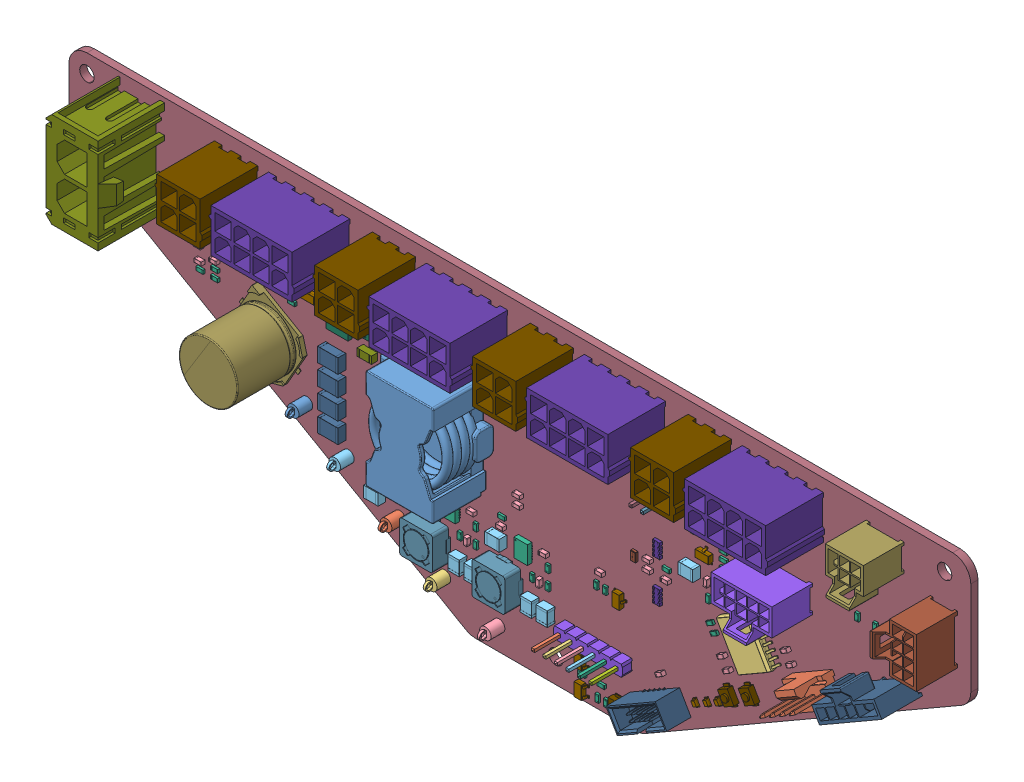
SolidWorks assembly zaphod-controller, configuration Default. Lengths in mm.
Overall size (199.92 69.34 18.57).
449 component instances, 49 part files, 0 mates.
Components (placement in the parent):
- PKMCS0909E4000-1: PKMCS0909E4000 [Default] at (113.5 -47 -0.05) x (-1 0 0) z (0 -1 0) size (9 1.9 9)
  - COMPOUND-1: COMPOUND [Default] at origin size (9 1.9 9)
- MOLEX_47053-1000-1: MOLEX_47053-1000 [Default] at (166.5524 -41.075 4.15) x (0.866025 0.5 0) z (0.5 -0.866025 0) size (10.2 13.5 5.84)
  - SOLID-1: SOLID [Default] at origin size (10.2 13.5 5.84)
- SOIC127P1032X265-16L87-1: SOIC127P1032X265-16L87 [Default] at (151.3126 -39.0334 1.65) x (0.5 -0.866025 0) z (0 0 1) size (10.08 10.17 2)
  - COMPOUND_2-1: COMPOUND_2 [Default] at origin size (10.08 10.17 2)
- CAPC1608X90-1: CAPC1608X90 [Default] at (147.0091 -44.05 -0.05) x (0 -1 0) z (0 0 -1) size (1.6 0.8 0.9)
  - COMPOUND_3-1: COMPOUND_3 [Default] at origin size (1.6 0.8 0.9)
- CAPC1608X90-2: CAPC1608X90 [Default] at (147.1 -51.575 -0.05) x (0 -1 0) z (0 0 -1) size (1.6 0.8 0.9)
  - COMPOUND_3-1: COMPOUND_3 [Default] at origin size (1.6 0.8 0.9)
- CAPC1608X90-3: CAPC1608X90 [Default] at (134.6 -51.575 -0.05) x (0 -1 0) z (0 0 -1) size (1.6 0.8 0.9)
  - COMPOUND_3-1: COMPOUND_3 [Default] at origin size (1.6 0.8 0.9)
- CAPC1608X90-4: CAPC1608X90 [Default] at (134.6 -45.075 -0.05) x (0 -1 0) z (0 0 -1) size (1.6 0.8 0.9)
  - COMPOUND_3-1: COMPOUND_3 [Default] at origin size (1.6 0.8 0.9)
- CAPC1608X90-5: CAPC1608X90 [Default] at (145.2978 -44.8154 1.65) x (0.866025 0.5 0) z (0 0 1) size (1.6 0.8 0.9)
  - COMPOUND_3-1: COMPOUND_3 [Default] at origin size (1.6 0.8 0.9)
- CAPC1608X90-6: CAPC1608X90 [Default] at (160.5774 -38.8805 1.65) x (-0.866025 -0.5 0) z (0 0 1) size (1.6 0.8 0.9)
  - COMPOUND_3-1: COMPOUND_3 [Default] at origin size (1.6 0.8 0.9)
- CAPC3225X170-1: CAPC3225X170 [Default] at (153.35 -43.55 -0.05) x (0 -1 0) z (0 0 -1) size (3.2 2.5 1.7)
  - COMPOUND_4-1: COMPOUND_4 [Default] at origin size (3.2 2.5 1.7)
- CAPC3225X170-2: CAPC3225X170 [Default] at (131.85 -44.325 -0.05) x (0 -1 0) z (0 0 -1) size (3.2 2.5 1.7)
  - COMPOUND_4-1: COMPOUND_4 [Default] at origin size (3.2 2.5 1.7)
- RESC1608X50-1: RESC1608X50 [Default] at (157.1 -45.05 -0.05) x (1 0 0) z (0 0 -1) size (1.6 0.8 0.5)
  - COMPOUND_5-1: COMPOUND_5 [Default] at origin size (1.6 0.8 0.5)
- RESC1608X50-2: RESC1608X50 [Default] at (156.5275 -31.8657 1.65) x (-0.866025 -0.5 0) z (0 0 1) size (1.6 0.8 0.5)
  - COMPOUND_5-1: COMPOUND_5 [Default] at origin size (1.6 0.8 0.5)
- RESC1608X50-3: RESC1608X50 [Default] at (157.1 -43.3 -0.05) x (1 0 0) z (0 0 -1) size (1.6 0.8 0.5)
  - COMPOUND_5-1: COMPOUND_5 [Default] at origin size (1.6 0.8 0.5)
- RESC1608X50-4: RESC1608X50 [Default] at (157.4525 -33.4678 1.65) x (-0.866025 -0.5 0) z (0 0 1) size (1.6 0.8 0.5)
  - COMPOUND_5-1: COMPOUND_5 [Default] at origin size (1.6 0.8 0.5)
- SOP65P780X200-24L40-1: SOP65P780X200-24L40 [Default] at (140.85 -47.8 -0.25) x (1 0 0) z (0 1 0) size (7.9 2.02 8.63)
  - SOLID_2-1: SOLID_2 [Default] at origin size (7.9 2.02 8.63)
- MOLEX_NANOFIT_1053101110-1: MOLEX_NANOFIT_1053101110 [Default] at (158.2 -24.35 6.5) x (-1 0 0) z (0 0 1) size (13.44 8.86 13.71)
  - SOLID_3-1: SOLID_3 [Default] at origin size (13.44 8.86 13.71)
- SOT95P240X110-3L16-1: SOT95P240X110-3L16 [Default] at (179 -22.5 -0.05) x (0 1 0) z (0 0 -1) size (2.91 3.01 1.23)
  - COMPOUND_6-1: COMPOUND_6 [Default] at origin size (2.91 3.01 1.23)
- RESC1608X50-5: RESC1608X50 [Default] at (182.7 -19.3 -0.05) x (-1 0 0) z (0 0 -1) size (1.6 0.8 0.5)
  - COMPOUND_5-1: COMPOUND_5 [Default] at origin size (1.6 0.8 0.5)
- MOLEX_NANOFIT_1053091106-1: MOLEX_NANOFIT_1053091106 [Default] at (181.5175 -33.225 6.5) x (0.866025 0.5 0) z (0 0 1) size (15.94 6.34 13.71)
  - SOLID_4-1: SOLID_4 [Default] at origin size (15.94 6.34 13.71)
- MOLEX_NANOFIT_1053101108-1: MOLEX_NANOFIT_1053101108 [Default] at (194.05 -16.05 6.55) x (0 1 0) z (0 0 1) size (10.94 8.84 13.71)
  - SOLID_5-1: SOLID_5 [Default] at origin size (10.94 8.84 13.71)
- MOLEX_NANOFIT_1053101106-1: MOLEX_NANOFIT_1053101106 [Default] at (181 -6.25 6.5) x (-1 0 0) z (0 0 1) size (8.44 8.84 13.71)
  - SOLID_6-1: SOLID_6 [Default] at origin size (8.44 8.84 13.71)
- 61300211121-1: 61300211121 [Default] at (133.83 -18.6 2.65) x (1 0 0) z (0 -1 0) size (5.08 11.54 2.54)
  - SOLID_7-1: SOLID_7 [Default] at origin size (0.64 11.54 0.64)
  - SOLID_8-1: SOLID_8 [Default] at origin size (0.64 11.54 0.64)
  - SOLID_9-1: SOLID_9 [Default] at origin size (5.08 2.54 2.54)
- RESC1608X50-6: RESC1608X50 [Default] at (132.8 -34.6 1.65) x (-1 0 0) z (0 0 1) size (1.6 0.8 0.5)
  - COMPOUND_5-1: COMPOUND_5 [Default] at origin size (1.6 0.8 0.5)
- RESC1608X50-7: RESC1608X50 [Default] at (133.8 -21.4 1.65) x (-1 0 0) z (0 0 1) size (1.6 0.8 0.5)
  - COMPOUND_5-1: COMPOUND_5 [Default] at origin size (1.6 0.8 0.5)
- RESC1608X50-8: RESC1608X50 [Default] at (57.7 -27.2 -0.05) x (1 0 0) z (0 0 -1) size (1.6 0.8 0.5)
  - COMPOUND_5-1: COMPOUND_5 [Default] at origin size (1.6 0.8 0.5)
- MOLEX_SABRE_431600102-1: MOLEX_SABRE_431600102 [Default] at (15.5 -11.45 9.05) x (0 1 0) z (1 0 0) size (21.08 18.57 13.39)
  - SOLID_10-1: SOLID_10 [Default] at origin size (21.08 18.57 13.39)
- MOLEX_MICROFITJR_039281083-1: MOLEX_MICROFITJR_039281083 [Default] at (53.3 -7.5 1.65) x (-1 0 0) z (0 1 0) size (18.8 16.3 11)
  - SOLID_11-1: SOLID_11 [Default] at origin size (18.8 16.3 11)
- MOLEX_MICROFITJR_039281083-2: MOLEX_MICROFITJR_039281083 [Default] at (88.3 -7.5 1.65) x (-1 0 0) z (0 1 0) size (18.8 16.3 11)
  - SOLID_11-1: SOLID_11 [Default] at origin size (18.8 16.3 11)
- MOLEX_MICROFITJR_039281083-3: MOLEX_MICROFITJR_039281083 [Default] at (123.3 -7.5 1.65) x (-1 0 0) z (0 1 0) size (18.8 16.3 11)
  - SOLID_11-1: SOLID_11 [Default] at origin size (18.8 16.3 11)
- MOLEX_MICROFITJR_039281083-4: MOLEX_MICROFITJR_039281083 [Default] at (158.3 -7.5 1.65) x (-1 0 0) z (0 1 0) size (18.8 16.3 11)
  - SOLID_11-1: SOLID_11 [Default] at origin size (18.8 16.3 11)
- MOLEX_MICROFITJR_039281043-1: MOLEX_MICROFITJR_039281043 [Default] at (37.1 -7.5 1.65) x (-1 0 0) z (0 1 0) size (10.4 16.3 11)
  - SOLID_12-1: SOLID_12 [Default] at origin size (10.4 16.3 11)
- MOLEX_MICROFITJR_039281043-2: MOLEX_MICROFITJR_039281043 [Default] at (72.1 -7.5 1.65) x (-1 0 0) z (0 1 0) size (10.4 16.3 11)
  - SOLID_12-1: SOLID_12 [Default] at origin size (10.4 16.3 11)
- MOLEX_MICROFITJR_039281043-3: MOLEX_MICROFITJR_039281043 [Default] at (107.1 -7.5 1.65) x (-1 0 0) z (0 1 0) size (10.4 16.3 11)
  - SOLID_12-1: SOLID_12 [Default] at origin size (10.4 16.3 11)
- MOLEX_MICROFITJR_039281043-4: MOLEX_MICROFITJR_039281043 [Default] at (142.1 -7.5 1.65) x (-1 0 0) z (0 1 0) size (10.4 16.3 11)
  - SOLID_12-1: SOLID_12 [Default] at origin size (10.4 16.3 11)
- PULSE_PA2050-1: PULSE_PA2050 [Default] at (84.85 -28.9 1.65) x (0 -1 0) z (-1 0 0) size (22.23 12.2 19.25)
  - SOLID_13-1: SOLID_13 [Default] at origin size (22.23 12.2 19.25)
- 61300611121-1: 61300611121 [Default] at (117.35 -57.1 2.65) x (1 0 0) z (0 -1 0) size (15.24 11.54 2.54)
  - SOLID_14-1: SOLID_14 [Default] at origin size (0.64 11.54 0.64)
  - SOLID_15-1: SOLID_15 [Default] at origin size (0.64 11.54 0.64)
  - SOLID_16-1: SOLID_16 [Default] at origin size (0.64 11.54 0.64)
  - SOLID_17-1: SOLID_17 [Default] at origin size (0.64 11.54 0.64)
  - SOLID_18-1: SOLID_18 [Default] at origin size (0.64 11.54 0.64)
  - SOLID_19-1: SOLID_19 [Default] at origin size (0.64 11.54 0.64)
  - SOLID_20-1: SOLID_20 [Default] at origin size (15.24 2.54 2.54)
- LEDC1608X80L40-1: LEDC1608X80L40 [Default] at (141.8 -55.6 1.75) x (-0.5 0.866025 0) z (0.866025 0.5 0) size (1.61 0.75 0.81)
  - COMPOUND_7-1: COMPOUND_7 [Default] at origin size (1.61 0.75 0.81)
- LEDC1608X80L40-2: LEDC1608X80L40 [Default] at (139.2 -57 1.75) x (-0.5 0.866025 0) z (0.866025 0.5 0) size (1.61 0.75 0.81)
  - COMPOUND_7-1: COMPOUND_7 [Default] at origin size (1.61 0.75 0.81)
- LEDC1608X80L40-3: LEDC1608X80L40 [Default] at (144.2 -54.3 1.75) x (-0.5 0.866025 0) z (0.866025 0.5 0) size (1.61 0.75 0.81)
  - COMPOUND_7-1: COMPOUND_7 [Default] at origin size (1.61 0.75 0.81)
- SOT95P240X110-3L16-2: SOT95P240X110-3L16 [Default] at (54.05 -21.3 1.65) x (0 -1 0) z (0 0 1) size (2.91 3.01 1.23)
  - COMPOUND_6-1: COMPOUND_6 [Default] at origin size (2.91 3.01 1.23)
- CAPC1608X90-7: CAPC1608X90 [Default] at (169.2907 -8.1731 -0.05) x (-1 0 0) z (0 0 -1) size (1.6 0.8 0.9)
  - COMPOUND_3-1: COMPOUND_3 [Default] at origin size (1.6 0.8 0.9)
- CAPC3225X170-3: CAPC3225X170 [Default] at (95.5 -47.25 1.65) size (3.2 2.5 1.7)
  - COMPOUND_4-1: COMPOUND_4 [Default] at origin size (3.2 2.5 1.7)
- CAPC4532X180-1: CAPC4532X180 [Default] at (59.2 -44 1.65) size (4.5 3.2 1.8)
  - COMPOUND_8-1: COMPOUND_8 [Default] at origin size (4.5 3.2 1.8)
- CAPC4532X180-2: CAPC4532X180 [Default] at (59.2 -39.5 1.65) size (4.5 3.2 1.8)
  - COMPOUND_8-1: COMPOUND_8 [Default] at origin size (4.5 3.2 1.8)
- CAPC1608X90-8: CAPC1608X90 [Default] at (96.275 -44.5 1.65) x (-1 0 0) z (0 0 1) size (1.6 0.8 0.9)
  - COMPOUND_3-1: COMPOUND_3 [Default] at origin size (1.6 0.8 0.9)
- CAPC4532X180-3: CAPC4532X180 [Default] at (59.2 -35 1.65) size (4.5 3.2 1.8)
  - COMPOUND_8-1: COMPOUND_8 [Default] at origin size (4.5 3.2 1.8)
- CAPC4532X180-4: CAPC4532X180 [Default] at (59.2 -30.5 1.65) size (4.5 3.2 1.8)
  - COMPOUND_8-1: COMPOUND_8 [Default] at origin size (4.5 3.2 1.8)
- CAPC1608X90-9: CAPC1608X90 [Default] at (32.7 -25.25 1.65) x (-1 0 0) z (0 0 1) size (1.6 0.8 0.9)
  - COMPOUND_3-1: COMPOUND_3 [Default] at origin size (1.6 0.8 0.9)
- CAPC1608X90-10: CAPC1608X90 [Default] at (105.725 -45 1.65) x (-1 0 0) z (0 0 1) size (1.6 0.8 0.9)
  - COMPOUND_3-1: COMPOUND_3 [Default] at origin size (1.6 0.8 0.9)
- CAPC1608X90-11: CAPC1608X90 [Default] at (29.2 -16.25 1.65) size (1.6 0.8 0.9)
  - COMPOUND_3-1: COMPOUND_3 [Default] at origin size (1.6 0.8 0.9)
- CAPC1608X90-12: CAPC1608X90 [Default] at (29.45 -27 1.65) size (1.6 0.8 0.9)
  - COMPOUND_3-1: COMPOUND_3 [Default] at origin size (1.6 0.8 0.9)
- CAPC1608X90-13: CAPC1608X90 [Default] at (104.75 -51 1.65) x (0 1 0) z (0 0 1) size (1.6 0.8 0.9)
  - COMPOUND_3-1: COMPOUND_3 [Default] at origin size (1.6 0.8 0.9)
- CAPC3225X170-4: CAPC3225X170 [Default] at (103 -56 1.65) x (0 -1 0) z (0 0 1) size (3.2 2.5 1.7)
  - COMPOUND_4-1: COMPOUND_4 [Default] at origin size (3.2 2.5 1.7)
- CAPC1608X90-14: CAPC1608X90 [Default] at (29.2 -24 1.65) x (-1 0 0) z (0 0 1) size (1.6 0.8 0.9)
  - COMPOUND_3-1: COMPOUND_3 [Default] at origin size (1.6 0.8 0.9)
- CAPC3225X170-5: CAPC3225X170 [Default] at (106.5 -56 1.65) x (0 -1 0) z (0 0 1) size (3.2 2.5 1.7)
  - COMPOUND_4-1: COMPOUND_4 [Default] at origin size (3.2 2.5 1.7)
- CAPC1608X90-15: CAPC1608X90 [Default] at (29.2 -22.25 1.65) x (-1 0 0) z (0 0 1) size (1.6 0.8 0.9)
  - COMPOUND_3-1: COMPOUND_3 [Default] at origin size (1.6 0.8 0.9)
- CAPC2012X110-1: CAPC2012X110 [Default] at (41.1 -25.3 -0.05) x (1 0 0) z (0 0 -1) size (2 1.2 1.1)
  - COMPOUND_9-1: COMPOUND_9 [Default] at origin size (2 1.2 1.1)
- CAPC2012X110-2: CAPC2012X110 [Default] at (49.8 -17.05 1.65) x (-1 0 0) z (0 0 1) size (2 1.2 1.1)
  - COMPOUND_9-1: COMPOUND_9 [Default] at origin size (2 1.2 1.1)
- CAPC3225X170-6: CAPC3225X170 [Default] at (79.5 -47.25 1.65) size (3.2 2.5 1.7)
  - COMPOUND_4-1: COMPOUND_4 [Default] at origin size (3.2 2.5 1.7)
- CAPC2012X110-3: CAPC2012X110 [Default] at (55.3 -17.05 1.65) x (0 -1 0) z (0 0 1) size (2 1.2 1.1)
  - COMPOUND_9-1: COMPOUND_9 [Default] at origin size (2 1.2 1.1)
- CAPC1608X90-16: CAPC1608X90 [Default] at (80.275 -44.5 1.65) x (-1 0 0) z (0 0 1) size (1.6 0.8 0.9)
  - COMPOUND_3-1: COMPOUND_3 [Default] at origin size (1.6 0.8 0.9)
- CAPC1608X90-17: CAPC1608X90 [Default] at (89.725 -45 1.65) x (-1 0 0) z (0 0 1) size (1.6 0.8 0.9)
  - COMPOUND_3-1: COMPOUND_3 [Default] at origin size (1.6 0.8 0.9)
- CAPC1608X90-18: CAPC1608X90 [Default] at (88.75 -51 1.65) x (0 1 0) z (0 0 1) size (1.6 0.8 0.9)
  - COMPOUND_3-1: COMPOUND_3 [Default] at origin size (1.6 0.8 0.9)
- CAPC3225X170-7: CAPC3225X170 [Default] at (90.5 -56 1.65) x (0 -1 0) z (0 0 1) size (3.2 2.5 1.7)
  - COMPOUND_4-1: COMPOUND_4 [Default] at origin size (3.2 2.5 1.7)
- CAPC3225X170-8: CAPC3225X170 [Default] at (68.65 -51.8 1.65) x (-1 0 0) z (0 0 1) size (3.2 2.5 1.7)
  - COMPOUND_4-1: COMPOUND_4 [Default] at origin size (3.2 2.5 1.7)
- CAPC3225X170-9: CAPC3225X170 [Default] at (87 -56 1.65) x (0 -1 0) z (0 0 1) size (3.2 2.5 1.7)
  - COMPOUND_4-1: COMPOUND_4 [Default] at origin size (3.2 2.5 1.7)
- CAPC1608X90-19: CAPC1608X90 [Default] at (103.8 -20 1.65) x (-1 0 0) z (0 0 1) size (1.6 0.8 0.9)
  - COMPOUND_3-1: COMPOUND_3 [Default] at origin size (1.6 0.8 0.9)
- CAPC1608X90-20: CAPC1608X90 [Default] at (128 -25.5 -0.05) x (0 1 0) z (0 0 -1) size (1.6 0.8 0.9)
  - COMPOUND_3-1: COMPOUND_3 [Default] at origin size (1.6 0.8 0.9)
- CAPC1608X90-21: CAPC1608X90 [Default] at (100 -36.6 1.65) x (-1 0 0) z (0 0 1) size (1.6 0.8 0.9)
  - COMPOUND_3-1: COMPOUND_3 [Default] at origin size (1.6 0.8 0.9)
- CAPC1608X90-22: CAPC1608X90 [Default] at (129.75 -25.5 -0.05) x (0 1 0) z (0 0 -1) size (1.6 0.8 0.9)
  - COMPOUND_3-1: COMPOUND_3 [Default] at origin size (1.6 0.8 0.9)
- CAPC1608X90-23: CAPC1608X90 [Default] at (131.6 -55.1 1.65) x (0.866025 0.5 0) z (0 0 1) size (1.6 0.8 0.9)
  - COMPOUND_3-1: COMPOUND_3 [Default] at origin size (1.6 0.8 0.9)
- CAPC1608X90-24: CAPC1608X90 [Default] at (146.5478 -46.9805 1.65) x (0.866025 0.5 0) z (0 0 1) size (1.6 0.8 0.9)
  - COMPOUND_3-1: COMPOUND_3 [Default] at origin size (1.6 0.8 0.9)
- CAPC1608X90-25: CAPC1608X90 [Default] at (123.6 -34.9 -0.05) x (-1 0 0) z (0 0 -1) size (1.6 0.8 0.9)
  - COMPOUND_3-1: COMPOUND_3 [Default] at origin size (1.6 0.8 0.9)
- CAPC1608X90-26: CAPC1608X90 [Default] at (123.6 -29.6 -0.05) x (1 0 0) z (0 0 -1) size (1.6 0.8 0.9)
  - COMPOUND_3-1: COMPOUND_3 [Default] at origin size (1.6 0.8 0.9)
- CAPC1608X90-27: CAPC1608X90 [Default] at (118.5 -21.6 1.65) size (1.6 0.8 0.9)
  - COMPOUND_3-1: COMPOUND_3 [Default] at origin size (1.6 0.8 0.9)
- CAPC1608X90-28: CAPC1608X90 [Default] at (103.8 -21.8 1.65) x (-1 0 0) z (0 0 1) size (1.6 0.8 0.9)
  - COMPOUND_3-1: COMPOUND_3 [Default] at origin size (1.6 0.8 0.9)
- CAPC1608X90-29: CAPC1608X90 [Default] at (100 -38.6 1.65) x (-1 0 0) z (0 0 1) size (1.6 0.8 0.9)
  - COMPOUND_3-1: COMPOUND_3 [Default] at origin size (1.6 0.8 0.9)
- CAPC1608X90-30: CAPC1608X90 [Default] at (124.5 -25.5 -0.05) x (0 1 0) z (0 0 -1) size (1.6 0.8 0.9)
  - COMPOUND_3-1: COMPOUND_3 [Default] at origin size (1.6 0.8 0.9)
- CAPC1608X90-31: CAPC1608X90 [Default] at (118.2 -42.4 1.65) x (-1 0 0) z (0 0 1) size (1.6 0.8 0.9)
  - COMPOUND_3-1: COMPOUND_3 [Default] at origin size (1.6 0.8 0.9)
- CAPC1608X90-32: CAPC1608X90 [Default] at (126.25 -25.5 -0.05) x (0 1 0) z (0 0 -1) size (1.6 0.8 0.9)
  - COMPOUND_3-1: COMPOUND_3 [Default] at origin size (1.6 0.8 0.9)
- CAPC1608X90-33: CAPC1608X90 [Default] at (128.8 -36.6 1.65) size (1.6 0.8 0.9)
  - COMPOUND_3-1: COMPOUND_3 [Default] at origin size (1.6 0.8 0.9)
- CAPC1608X90-34: CAPC1608X90 [Default] at (128.8 -34.6 1.65) size (1.6 0.8 0.9)
  - COMPOUND_3-1: COMPOUND_3 [Default] at origin size (1.6 0.8 0.9)
- CAPC1608X90-35: CAPC1608X90 [Default] at (30 -11.009 -0.05) x (-1 0 0) z (0 0 -1) size (1.6 0.8 0.9)
  - COMPOUND_3-1: COMPOUND_3 [Default] at origin size (1.6 0.8 0.9)
- CAPC1608X90-36: CAPC1608X90 [Default] at (64.9267 -11 -0.05) x (-1 0 0) z (0 0 -1) size (1.6 0.8 0.9)
  - COMPOUND_3-1: COMPOUND_3 [Default] at origin size (1.6 0.8 0.9)
- CAPC1608X90-37: CAPC1608X90 [Default] at (100 -11 -0.05) x (-1 0 0) z (0 0 -1) size (1.6 0.8 0.9)
  - COMPOUND_3-1: COMPOUND_3 [Default] at origin size (1.6 0.8 0.9)
- CAPC1608X90-38: CAPC1608X90 [Default] at (134.8 -11 -0.05) x (-1 0 0) z (0 0 -1) size (1.6 0.8 0.9)
  - COMPOUND_3-1: COMPOUND_3 [Default] at origin size (1.6 0.8 0.9)
- CAPC1608X90-39: CAPC1608X90 [Default] at (90.298 -35.5 -0.05) x (-1 0 0) z (0 0 -1) size (1.6 0.8 0.9)
  - COMPOUND_3-1: COMPOUND_3 [Default] at origin size (1.6 0.8 0.9)
- CAPC1608X90-40: CAPC1608X90 [Default] at (140.602 -20.7 -0.05) x (1 0 0) z (0 0 -1) size (1.6 0.8 0.9)
  - COMPOUND_3-1: COMPOUND_3 [Default] at origin size (1.6 0.8 0.9)
- CAPC1608X90-41: CAPC1608X90 [Default] at (46.9727 -15.598 -0.05) x (0 -1 0) z (0 0 -1) size (1.6 0.8 0.9)
  - COMPOUND_3-1: COMPOUND_3 [Default] at origin size (1.6 0.8 0.9)
- CAPC1608X90-42: CAPC1608X90 [Default] at (117 -15.598 -0.05) x (0 -1 0) z (0 0 -1) size (1.6 0.8 0.9)
  - COMPOUND_3-1: COMPOUND_3 [Default] at origin size (1.6 0.8 0.9)
- CAPC1608X90-43: CAPC1608X90 [Default] at (81.9353 -15.5817 -0.05) x (0 -1 0) z (0 0 -1) size (1.6 0.8 0.9)
  - COMPOUND_3-1: COMPOUND_3 [Default] at origin size (1.6 0.8 0.9)
- CAPC1608X90-44: CAPC1608X90 [Default] at (152 -15.6 -0.05) x (0 -1 0) z (0 0 -1) size (1.6 0.8 0.9)
  - COMPOUND_3-1: COMPOUND_3 [Default] at origin size (1.6 0.8 0.9)
- CAPC1608X90-45: CAPC1608X90 [Default] at (187.9 -12.5 -0.05) x (1 0 0) z (0 0 -1) size (1.6 0.8 0.9)
  - COMPOUND_3-1: COMPOUND_3 [Default] at origin size (1.6 0.8 0.9)
- CAPC1608X90-46: CAPC1608X90 [Default] at (187.9 -14.2 -0.05) x (1 0 0) z (0 0 -1) size (1.6 0.8 0.9)
  - COMPOUND_3-1: COMPOUND_3 [Default] at origin size (1.6 0.8 0.9)
- CAPC1608X90-47: CAPC1608X90 [Default] at (187.9 -15.9 -0.05) x (1 0 0) z (0 0 -1) size (1.6 0.8 0.9)
  - COMPOUND_3-1: COMPOUND_3 [Default] at origin size (1.6 0.8 0.9)
- CAPC1608X90-48: CAPC1608X90 [Default] at (187.9 -17.6 -0.05) x (1 0 0) z (0 0 -1) size (1.6 0.8 0.9)
  - COMPOUND_3-1: COMPOUND_3 [Default] at origin size (1.6 0.8 0.9)
- CAPC1608X90-49: CAPC1608X90 [Default] at (187.9 -19.3 -0.05) x (1 0 0) z (0 0 -1) size (1.6 0.8 0.9)
  - COMPOUND_3-1: COMPOUND_3 [Default] at origin size (1.6 0.8 0.9)
- CAPC1608X90-50: CAPC1608X90 [Default] at (159.3274 -36.7154 1.65) x (-0.866025 -0.5 0) z (0 0 1) size (1.6 0.8 0.9)
  - COMPOUND_3-1: COMPOUND_3 [Default] at origin size (1.6 0.8 0.9)
- CAPC1608X90-51: CAPC1608X90 [Default] at (187.8692 -27.1 -0.05) x (1 0 0) z (0 0 -1) size (1.6 0.8 0.9)
  - COMPOUND_3-1: COMPOUND_3 [Default] at origin size (1.6 0.8 0.9)
- CAPC1608X90-52: CAPC1608X90 [Default] at (187.8442 -25.4 -0.05) x (1 0 0) z (0 0 -1) size (1.6 0.8 0.9)
  - COMPOUND_3-1: COMPOUND_3 [Default] at origin size (1.6 0.8 0.9)
- CAPC1608X90-53: CAPC1608X90 [Default] at (187.8692 -23.7 -0.05) x (1 0 0) z (0 0 -1) size (1.6 0.8 0.9)
  - COMPOUND_3-1: COMPOUND_3 [Default] at origin size (1.6 0.8 0.9)
- CAPC1608X90-54: CAPC1608X90 [Default] at (187.9 -22 -0.05) x (1 0 0) z (0 0 -1) size (1.6 0.8 0.9)
  - COMPOUND_3-1: COMPOUND_3 [Default] at origin size (1.6 0.8 0.9)
- CAPC1608X90-55: CAPC1608X90 [Default] at (132.775 -36.6 1.65) size (1.6 0.8 0.9)
  - COMPOUND_3-1: COMPOUND_3 [Default] at origin size (1.6 0.8 0.9)
- CAPC1608X90-56: CAPC1608X90 [Default] at (57.7 -29.1 -0.05) x (-1 0 0) z (0 0 -1) size (1.6 0.8 0.9)
  - COMPOUND_3-1: COMPOUND_3 [Default] at origin size (1.6 0.8 0.9)
- CAPC3225X170-10: CAPC3225X170 [Default] at (138.4 -31.6 1.65) size (3.2 2.5 1.7)
  - COMPOUND_4-1: COMPOUND_4 [Default] at origin size (3.2 2.5 1.7)
- CAPC1608X90-57: CAPC1608X90 [Default] at (133.8 -23.1 1.65) size (1.6 0.8 0.9)
  - COMPOUND_3-1: COMPOUND_3 [Default] at origin size (1.6 0.8 0.9)
- CAPC1608X90-58: CAPC1608X90 [Default] at (141.9 -32.375 1.65) x (0 1 0) z (0 0 1) size (1.6 0.8 0.9)
  - COMPOUND_3-1: COMPOUND_3 [Default] at origin size (1.6 0.8 0.9)
- SOT95P240X110-3L16-3: SOT95P240X110-3L16 [Default] at (169.2907 -11.3731 -0.05) x (0 1 0) z (0 0 -1) size (2.91 3.01 1.23)
  - COMPOUND_6-1: COMPOUND_6 [Default] at origin size (2.91 3.01 1.23)
- SOT95P240X110-3L16-4: SOT95P240X110-3L16 [Default] at (32.95 -15.25 1.65) x (-1 0 0) z (0 0 1) size (2.91 3.01 1.23)
  - COMPOUND_6-1: COMPOUND_6 [Default] at origin size (2.91 3.01 1.23)
- SOT95P240X110-3L16-5: SOT95P240X110-3L16 [Default] at (42 -15.598 -0.05) x (0 1 0) z (0 0 -1) size (2.91 3.01 1.23)
  - COMPOUND_6-1: COMPOUND_6 [Default] at origin size (2.91 3.01 1.23)
- SOT95P240X110-3L16-6: SOT95P240X110-3L16 [Default] at (112.2 -15.6 -0.05) x (0 1 0) z (0 0 -1) size (2.91 3.01 1.23)
  - COMPOUND_6-1: COMPOUND_6 [Default] at origin size (2.91 3.01 1.23)
- SOT95P240X110-3L16-7: SOT95P240X110-3L16 [Default] at (77 -15.6 -0.05) x (0 1 0) z (0 0 -1) size (2.91 3.01 1.23)
  - COMPOUND_6-1: COMPOUND_6 [Default] at origin size (2.91 3.01 1.23)
- SOT95P240X110-3L16-8: SOT95P240X110-3L16 [Default] at (147.2 -15.6 -0.05) x (0 1 0) z (0 0 -1) size (2.91 3.01 1.23)
  - COMPOUND_6-1: COMPOUND_6 [Default] at origin size (2.91 3.01 1.23)
- DO-215AD-1: DO-215AD [Default] at (49.2 -15.598 -0.05) x (0 -1 0) z (0 0 -1) size (3.85 1.7 1.35)
  - COMPOUND_10-1: COMPOUND_10 [Default] at origin size (3.85 1.7 1.35)
- DO-215AD-2: DO-215AD [Default] at (84.2 -15.6 -0.05) x (0 -1 0) z (0 0 -1) size (3.85 1.7 1.35)
  - COMPOUND_10-1: COMPOUND_10 [Default] at origin size (3.85 1.7 1.35)
- DO-215AD-3: DO-215AD [Default] at (119.2 -15.598 -0.05) x (0 -1 0) z (0 0 -1) size (3.85 1.7 1.35)
  - COMPOUND_10-1: COMPOUND_10 [Default] at origin size (3.85 1.7 1.35)
- DO-215AD-4: DO-215AD [Default] at (154.2 -15.6 -0.05) x (0 -1 0) z (0 0 -1) size (3.85 1.7 1.35)
  - COMPOUND_10-1: COMPOUND_10 [Default] at origin size (3.85 1.7 1.35)
- SOT95P240X110-3L16-9: SOT95P240X110-3L16 [Default] at (179 -12.5 -0.05) x (0 1 0) z (0 0 -1) size (2.91 3.01 1.23)
  - COMPOUND_6-1: COMPOUND_6 [Default] at origin size (2.91 3.01 1.23)
- SOT95P240X110-3L16-10: SOT95P240X110-3L16 [Default] at (175.1 -12.5 -0.05) x (0 1 0) z (0 0 -1) size (2.91 3.01 1.23)
  - COMPOUND_6-1: COMPOUND_6 [Default] at origin size (2.91 3.01 1.23)
- SOT95P240X110-3L16-11: SOT95P240X110-3L16 [Default] at (175.1 -17.6 -0.05) x (0 -1 0) z (0 0 -1) size (2.91 3.01 1.23)
  - COMPOUND_6-1: COMPOUND_6 [Default] at origin size (2.91 3.01 1.23)
- SOT95P240X110-3L16-12: SOT95P240X110-3L16 [Default] at (179 -17.6 -0.05) x (0 -1 0) z (0 0 -1) size (2.91 3.01 1.23)
  - COMPOUND_6-1: COMPOUND_6 [Default] at origin size (2.91 3.01 1.23)
- SOT95P240X110-3L16-13: SOT95P240X110-3L16 [Default] at (171.2 -17.6 -0.05) x (0 -1 0) z (0 0 -1) size (2.91 3.01 1.23)
  - COMPOUND_6-1: COMPOUND_6 [Default] at origin size (2.91 3.01 1.23)
- SOT95P240X110-3L16-14: SOT95P240X110-3L16 [Default] at (179 -27.8 -0.05) x (0 -1 0) z (0 0 -1) size (2.91 3.01 1.23)
  - COMPOUND_6-1: COMPOUND_6 [Default] at origin size (2.91 3.01 1.23)
- SOT95P240X110-3L16-15: SOT95P240X110-3L16 [Default] at (175.1 -27.8 -0.05) x (0 -1 0) z (0 0 -1) size (2.91 3.01 1.23)
  - COMPOUND_6-1: COMPOUND_6 [Default] at origin size (2.91 3.01 1.23)
- SOT95P240X110-3L16-16: SOT95P240X110-3L16 [Default] at (175.1 -22.5 -0.05) x (0 1 0) z (0 0 -1) size (2.91 3.01 1.23)
  - COMPOUND_6-1: COMPOUND_6 [Default] at origin size (2.91 3.01 1.23)
- SOT95P240X110-3L16-17: SOT95P240X110-3L16 [Default] at (141.5 -27.4 1.65) x (0 -1 0) z (0 0 1) size (2.91 3.01 1.23)
  - COMPOUND_6-1: COMPOUND_6 [Default] at origin size (2.91 3.01 1.23)
- 3225M_POLYFUSE-1: 3225M_POLYFUSE [Default] at (145.4685 -31.6 1.65) x (-1 0 0) z (0 1 0) size (3.22 0.68 2.58)
  - COMPOUND_11-1: COMPOUND_11 [Default] at origin size (3.22 0.68 2.58)
- INDM7300x7300x355-1: INDM7300x7300x355 [Default] at (97 -54 2.65) x (-1 0 0) z (0 1 0) size (7.3 4.01 7.3)
  - COMPOUND_12-1: COMPOUND_12 [Default] at origin size (7.3 4.01 7.3)
- INDM7300x7300x355-2: INDM7300x7300x355 [Default] at (81 -54 2.65) x (-1 0 0) z (0 1 0) size (7.3 4.01 7.3)
  - COMPOUND_12-1: COMPOUND_12 [Default] at origin size (7.3 4.01 7.3)
- SON127P490X575X90-9T313X381-1: SON127P490X575X90-9T313X381 [Default] at (60.4 -22.55 1.7) x (0 -1 0) z (0 0 1) size (6.01 4.9 0.95)
  - SOLID_21-1: SOLID_21 [Default] at origin size (6.01 4.9 0.95)
- SON127P490X575X90-9T313X381-2: SON127P490X575X90-9T313X381 [Default] at (68.65 -20.3 1.7) x (0 1 0) z (0 0 1) size (6.01 4.9 0.95)
  - SOLID_21-1: SOLID_21 [Default] at origin size (6.01 4.9 0.95)
- SOT95P240X110-3L16-18: SOT95P240X110-3L16 [Default] at (114 -66.9 1.65) size (2.91 3.01 1.23)
  - COMPOUND_6-1: COMPOUND_6 [Default] at origin size (2.91 3.01 1.23)
- SOT95P240X110-3L16-19: SOT95P240X110-3L16 [Default] at (114 -61.2 1.65) size (2.91 3.01 1.23)
  - COMPOUND_6-1: COMPOUND_6 [Default] at origin size (2.91 3.01 1.23)
- SOT95P240X110-3L16-20: SOT95P240X110-3L16 [Default] at (141.5 -23.1 1.65) x (0 -1 0) z (0 0 1) size (2.91 3.01 1.23)
  - COMPOUND_6-1: COMPOUND_6 [Default] at origin size (2.91 3.01 1.23)
- SOT95P240X110-3L16-21: SOT95P240X110-3L16 [Default] at (122.4 -45.4 1.65) x (-1 0 0) z (0 0 1) size (2.91 3.01 1.23)
  - COMPOUND_6-1: COMPOUND_6 [Default] at origin size (2.91 3.01 1.23)
- RESC1608X50-9: RESC1608X50 [Default] at (169.2907 -2.1731 -0.05) x (1 0 0) z (0 0 -1) size (1.6 0.8 0.5)
  - COMPOUND_5-1: COMPOUND_5 [Default] at origin size (1.6 0.8 0.5)
- RESC1608X50-10: RESC1608X50 [Default] at (169.2907 -4.1731 -0.05) x (-1 0 0) z (0 0 -1) size (1.6 0.8 0.5)
  - COMPOUND_5-1: COMPOUND_5 [Default] at origin size (1.6 0.8 0.5)
- RESC1608X50-11: RESC1608X50 [Default] at (169.2907 -6.1731 -0.05) x (1 0 0) z (0 0 -1) size (1.6 0.8 0.5)
  - COMPOUND_5-1: COMPOUND_5 [Default] at origin size (1.6 0.8 0.5)
- RESC1608X50-12: RESC1608X50 [Default] at (103 -51 1.65) x (0 -1 0) z (0 0 1) size (1.6 0.8 0.5)
  - COMPOUND_5-1: COMPOUND_5 [Default] at origin size (1.6 0.8 0.5)
- RESC1608X50-13: RESC1608X50 [Default] at (32.7 -21 1.65) x (-1 0 0) z (0 0 1) size (1.6 0.8 0.5)
  - COMPOUND_5-1: COMPOUND_5 [Default] at origin size (1.6 0.8 0.5)
- RESC1608X50-14: RESC1608X50 [Default] at (29.2 -19.75 1.65) size (1.6 0.8 0.5)
  - COMPOUND_5-1: COMPOUND_5 [Default] at origin size (1.6 0.8 0.5)
- RESC1608X50-15: RESC1608X50 [Default] at (96.275 -42.75 1.65) x (-1 0 0) z (0 0 1) size (1.6 0.8 0.5)
  - COMPOUND_5-1: COMPOUND_5 [Default] at origin size (1.6 0.8 0.5)
- RESC1608X50-16: RESC1608X50 [Default] at (106.5 -51 1.65) x (0 1 0) z (0 0 1) size (1.6 0.8 0.5)
  - COMPOUND_5-1: COMPOUND_5 [Default] at origin size (1.6 0.8 0.5)
- RESC1608X50-17: RESC1608X50 [Default] at (106.5 -47.5 1.65) x (0 1 0) z (0 0 1) size (1.6 0.8 0.5)
  - COMPOUND_5-1: COMPOUND_5 [Default] at origin size (1.6 0.8 0.5)
- RESC1608X50-18: RESC1608X50 [Default] at (32.7 -18 1.65) x (-1 0 0) z (0 0 1) size (1.6 0.8 0.5)
  - COMPOUND_5-1: COMPOUND_5 [Default] at origin size (1.6 0.8 0.5)
- RESC1608X50-19: RESC1608X50 [Default] at (29.2 -18 1.65) x (-1 0 0) z (0 0 1) size (1.6 0.8 0.5)
  - COMPOUND_5-1: COMPOUND_5 [Default] at origin size (1.6 0.8 0.5)
- RESC1608X50-20: RESC1608X50 [Default] at (32.7 -27 1.65) x (-1 0 0) z (0 0 1) size (1.6 0.8 0.5)
  - COMPOUND_5-1: COMPOUND_5 [Default] at origin size (1.6 0.8 0.5)
- RESC1608X50-21: RESC1608X50 [Default] at (29.45 -28.75 1.65) x (-1 0 0) z (0 0 1) size (1.6 0.8 0.5)
  - COMPOUND_5-1: COMPOUND_5 [Default] at origin size (1.6 0.8 0.5)
- RESC1608X50-22: RESC1608X50 [Default] at (32.7 -28.75 1.65) x (-1 0 0) z (0 0 1) size (1.6 0.8 0.5)
  - COMPOUND_5-1: COMPOUND_5 [Default] at origin size (1.6 0.8 0.5)
- RESC1608X50-23: RESC1608X50 [Default] at (41.1 -23.3 -0.05) x (-1 0 0) z (0 0 -1) size (1.6 0.8 0.5)
  - COMPOUND_5-1: COMPOUND_5 [Default] at origin size (1.6 0.8 0.5)
- RESC1608X50-24: RESC1608X50 [Default] at (53.05 -17.05 1.65) x (0 -1 0) z (0 0 1) size (1.6 0.8 0.5)
  - COMPOUND_5-1: COMPOUND_5 [Default] at origin size (1.6 0.8 0.5)
- RESC1608X50-25: RESC1608X50 [Default] at (49.8 -19.05 1.65) x (-1 0 0) z (0 0 1) size (1.6 0.8 0.5)
  - COMPOUND_5-1: COMPOUND_5 [Default] at origin size (1.6 0.8 0.5)
- RESC1608X50-26: RESC1608X50 [Default] at (87 -51 1.65) x (0 -1 0) z (0 0 1) size (1.6 0.8 0.5)
  - COMPOUND_5-1: COMPOUND_5 [Default] at origin size (1.6 0.8 0.5)
- RESC1608X50-27: RESC1608X50 [Default] at (55.2 -20.25 -0.05) x (0 -1 0) z (0 0 -1) size (1.6 0.8 0.5)
  - COMPOUND_5-1: COMPOUND_5 [Default] at origin size (1.6 0.8 0.5)
- RESC1608X50-28: RESC1608X50 [Default] at (49.8 -23.05 1.65) x (-1 0 0) z (0 0 1) size (1.6 0.8 0.5)
  - COMPOUND_5-1: COMPOUND_5 [Default] at origin size (1.6 0.8 0.5)
- RESC1608X50-29: RESC1608X50 [Default] at (49.8 -21.3 1.65) x (-1 0 0) z (0 0 1) size (1.6 0.8 0.5)
  - COMPOUND_5-1: COMPOUND_5 [Default] at origin size (1.6 0.8 0.5)
- RESC1608X50-30: RESC1608X50 [Default] at (49.8 -24.8 1.65) x (-1 0 0) z (0 0 1) size (1.6 0.8 0.5)
  - COMPOUND_5-1: COMPOUND_5 [Default] at origin size (1.6 0.8 0.5)
- RESC3216X140-1: RESC3216X140 [Default] at (66.9 -26.05 1.65) x (-1 0 0) z (0 0 1) size (3.2 1.6 1.4)
  - COMPOUND_13-1: COMPOUND_13 [Default] at origin size (3.2 1.6 1.4)
- RESC1608X50-31: RESC1608X50 [Default] at (80.275 -42.75 1.65) x (-1 0 0) z (0 0 1) size (1.6 0.8 0.5)
  - COMPOUND_5-1: COMPOUND_5 [Default] at origin size (1.6 0.8 0.5)
- RESC1608X50-32: RESC1608X50 [Default] at (90.5 -51 1.65) x (0 1 0) z (0 0 1) size (1.6 0.8 0.5)
  - COMPOUND_5-1: COMPOUND_5 [Default] at origin size (1.6 0.8 0.5)
- RESC1608X50-33: RESC1608X50 [Default] at (90.5 -47.525 1.65) x (0 1 0) z (0 0 1) size (1.6 0.8 0.5)
  - COMPOUND_5-1: COMPOUND_5 [Default] at origin size (1.6 0.8 0.5)
- RESC1608X50-34: RESC1608X50 [Default] at (118.4 -64 1.65) x (-1 0 0) z (0 0 1) size (1.6 0.8 0.5)
  - COMPOUND_5-1: COMPOUND_5 [Default] at origin size (1.6 0.8 0.5)
- R_Array_Concave_4x060-1: R_Array_Concave_4x060 [Default] at (130.8 -40.6 1.65) x (0 -1 0) z (-1 0 0) size (3.2 0.65 1.6)
  - SOLID_22-1: SOLID_22 [Default] at origin size (3.2 0.65 1.6)
- RESC1608X50-35: RESC1608X50 [Default] at (143.3978 -41.5245 1.65) x (-0.866025 -0.5 0) z (0 0 1) size (1.6 0.8 0.5)
  - COMPOUND_5-1: COMPOUND_5 [Default] at origin size (1.6 0.8 0.5)
- RESC1608X50-36: RESC1608X50 [Default] at (142.4978 -39.9657 1.65) x (-0.866025 -0.5 0) z (0 0 1) size (1.6 0.8 0.5)
  - COMPOUND_5-1: COMPOUND_5 [Default] at origin size (1.6 0.8 0.5)
- RESC1608X50-37: RESC1608X50 [Default] at (123.6 -36.6 -0.05) x (1 0 0) z (0 0 -1) size (1.6 0.8 0.5)
  - COMPOUND_5-1: COMPOUND_5 [Default] at origin size (1.6 0.8 0.5)
- RESC1608X50-38: RESC1608X50 [Default] at (179.1 -22.4 1.65) x (0 1 0) z (0 0 1) size (1.6 0.8 0.5)
  - COMPOUND_5-1: COMPOUND_5 [Default] at origin size (1.6 0.8 0.5)
- RESC1608X50-39: RESC1608X50 [Default] at (175.1 -22.5 1.65) x (0 -1 0) z (0 0 1) size (1.6 0.8 0.5)
  - COMPOUND_5-1: COMPOUND_5 [Default] at origin size (1.6 0.8 0.5)
- R_Array_Concave_4x060-2: R_Array_Concave_4x060 [Default] at (114.4 -18.6 1.65) x (-1 0 0) z (0 1 0) size (3.2 0.65 1.6)
  - SOLID_22-1: SOLID_22 [Default] at origin size (3.2 0.65 1.6)
- RESC1608X50-40: RESC1608X50 [Default] at (30 -12.8 -0.05) x (-1 0 0) z (0 0 -1) size (1.6 0.8 0.5)
  - COMPOUND_5-1: COMPOUND_5 [Default] at origin size (1.6 0.8 0.5)
- RESC1608X50-41: RESC1608X50 [Default] at (64.9267 -12.8 -0.05) x (-1 0 0) z (0 0 -1) size (1.6 0.8 0.5)
  - COMPOUND_5-1: COMPOUND_5 [Default] at origin size (1.6 0.8 0.5)
- RESC1608X50-42: RESC1608X50 [Default] at (99.9 -12.8 -0.05) x (-1 0 0) z (0 0 -1) size (1.6 0.8 0.5)
  - COMPOUND_5-1: COMPOUND_5 [Default] at origin size (1.6 0.8 0.5)
- RESC1608X50-43: RESC1608X50 [Default] at (134.8 -12.8 -0.05) x (-1 0 0) z (0 0 -1) size (1.6 0.8 0.5)
  - COMPOUND_5-1: COMPOUND_5 [Default] at origin size (1.6 0.8 0.5)
- RESC1608X50-44: RESC1608X50 [Default] at (46 -18.2 -0.05) x (-1 0 0) z (0 0 -1) size (1.6 0.8 0.5)
  - COMPOUND_5-1: COMPOUND_5 [Default] at origin size (1.6 0.8 0.5)
- RESC1608X50-45: RESC1608X50 [Default] at (81 -18.4 -0.05) x (-1 0 0) z (0 0 -1) size (1.6 0.8 0.5)
  - COMPOUND_5-1: COMPOUND_5 [Default] at origin size (1.6 0.8 0.5)
- RESC1608X50-46: RESC1608X50 [Default] at (115.9727 -18.4 -0.05) x (-1 0 0) z (0 0 -1) size (1.6 0.8 0.5)
  - COMPOUND_5-1: COMPOUND_5 [Default] at origin size (1.6 0.8 0.5)
- RESC1608X50-47: RESC1608X50 [Default] at (151 -18.4 -0.05) x (-1 0 0) z (0 0 -1) size (1.6 0.8 0.5)
  - COMPOUND_5-1: COMPOUND_5 [Default] at origin size (1.6 0.8 0.5)
- RESC1608X50-48: RESC1608X50 [Default] at (44.9727 -15.623 -0.05) x (0 -1 0) z (0 0 -1) size (1.6 0.8 0.5)
  - COMPOUND_5-1: COMPOUND_5 [Default] at origin size (1.6 0.8 0.5)
- RESC1608X50-49: RESC1608X50 [Default] at (80 -15.6 -0.05) x (0 -1 0) z (0 0 -1) size (1.6 0.8 0.5)
  - COMPOUND_5-1: COMPOUND_5 [Default] at origin size (1.6 0.8 0.5)
- RESC1608X50-50: RESC1608X50 [Default] at (114.9727 -15.598 -0.05) x (0 -1 0) z (0 0 -1) size (1.6 0.8 0.5)
  - COMPOUND_5-1: COMPOUND_5 [Default] at origin size (1.6 0.8 0.5)
- RESC1608X50-51: RESC1608X50 [Default] at (150.0554 -15.6 -0.05) x (0 -1 0) z (0 0 -1) size (1.6 0.8 0.5)
  - COMPOUND_5-1: COMPOUND_5 [Default] at origin size (1.6 0.8 0.5)
- R_Array_Concave_4x060-3: R_Array_Concave_4x060 [Default] at (182.7 -15.1 -0.05) x (0 -1 0) z (1 0 0) size (3.2 0.65 1.6)
  - SOLID_22-1: SOLID_22 [Default] at origin size (3.2 0.65 1.6)
- RESC1608X50-52: RESC1608X50 [Default] at (182.7 -27.1 -0.05) x (-1 0 0) z (0 0 -1) size (1.6 0.8 0.5)
  - COMPOUND_5-1: COMPOUND_5 [Default] at origin size (1.6 0.8 0.5)
- RESC1608X50-53: RESC1608X50 [Default] at (182.7 -25.4 -0.05) x (-1 0 0) z (0 0 -1) size (1.6 0.8 0.5)
  - COMPOUND_5-1: COMPOUND_5 [Default] at origin size (1.6 0.8 0.5)
- RESC1608X50-54: RESC1608X50 [Default] at (182.7442 -23.7 -0.05) x (-1 0 0) z (0 0 -1) size (1.6 0.8 0.5)
  - COMPOUND_5-1: COMPOUND_5 [Default] at origin size (1.6 0.8 0.5)
- RESC1608X50-55: RESC1608X50 [Default] at (182.7442 -22 -0.05) x (-1 0 0) z (0 0 -1) size (1.6 0.8 0.5)
  - COMPOUND_5-1: COMPOUND_5 [Default] at origin size (1.6 0.8 0.5)
- RESC1608X50-56: RESC1608X50 [Default] at (119.4 -66.9 1.65) x (0 1 0) z (0 0 1) size (1.6 0.8 0.5)
  - COMPOUND_5-1: COMPOUND_5 [Default] at origin size (1.6 0.8 0.5)
- RESC1608X50-57: RESC1608X50 [Default] at (117.5 -66.9 1.65) x (0 1 0) z (0 0 1) size (1.6 0.8 0.5)
  - COMPOUND_5-1: COMPOUND_5 [Default] at origin size (1.6 0.8 0.5)
- RESC1608X50-58: RESC1608X50 [Default] at (114.1 -64 1.65) size (1.6 0.8 0.5)
  - COMPOUND_5-1: COMPOUND_5 [Default] at origin size (1.6 0.8 0.5)
- R_Array_Concave_4x060-4: R_Array_Concave_4x060 [Default] at (130.8 -31.6 1.65) x (0 1 0) z (1 0 0) size (3.2 0.65 1.6)
  - SOLID_22-1: SOLID_22 [Default] at origin size (3.2 0.65 1.6)
- RESC1608X50-59: RESC1608X50 [Default] at (138.6 -23.9 1.65) x (0 -1 0) z (0 0 1) size (1.6 0.8 0.5)
  - COMPOUND_5-1: COMPOUND_5 [Default] at origin size (1.6 0.8 0.5)
- RESC1608X50-60: RESC1608X50 [Default] at (145.4685 -24.8 1.65) size (1.6 0.8 0.5)
  - COMPOUND_5-1: COMPOUND_5 [Default] at origin size (1.6 0.8 0.5)
- RESC1608X50-61: RESC1608X50 [Default] at (117.2 -45.3548 1.65) x (0 -1 0) z (0 0 1) size (1.6 0.8 0.5)
  - COMPOUND_5-1: COMPOUND_5 [Default] at origin size (1.6 0.8 0.5)
- RESC1608X50-62: RESC1608X50 [Default] at (119.2 -45.3548 1.65) x (0 -1 0) z (0 0 1) size (1.6 0.8 0.5)
  - COMPOUND_5-1: COMPOUND_5 [Default] at origin size (1.6 0.8 0.5)
- RESC1608X50-63: RESC1608X50 [Default] at (145.4685 -26.4833 1.65) x (-1 0 0) z (0 0 1) size (1.6 0.8 0.5)
  - COMPOUND_5-1: COMPOUND_5 [Default] at origin size (1.6 0.8 0.5)
- RESC1608X50-64: RESC1608X50 [Default] at (145.5 -23.1 1.65) size (1.6 0.8 0.5)
  - COMPOUND_5-1: COMPOUND_5 [Default] at origin size (1.6 0.8 0.5)
- RESC1608X50-65: RESC1608X50 [Default] at (145.4685 -28.2 1.65) x (-1 0 0) z (0 0 1) size (1.6 0.8 0.5)
  - COMPOUND_5-1: COMPOUND_5 [Default] at origin size (1.6 0.8 0.5)
- B3U-1000P-1: B3U-1000P [Default] at (122 -66.2 1.65) x (0 1 0) z (1 0 0) size (4 1.6 2.5)
  - SOLID_23-1: SOLID_23 [Default] at origin size (4 1.6 2.5)
- B3U-1000P-2: B3U-1000P [Default] at (151.4 -49.3 1.65) x (0.5 -0.866025 0) z (-0.866025 -0.5 0) size (4 1.6 2.5)
  - SOLID_23-1: SOLID_23 [Default] at origin size (4 1.6 2.5)
- B3U-1000P-3: B3U-1000P [Default] at (146.8 -51.8 1.65) x (0.5 -0.866025 0) z (-0.866025 -0.5 0) size (4 1.6 2.5)
  - SOLID_23-1: SOLID_23 [Default] at origin size (4 1.6 2.5)
- KEYSTONE_5115_BROWN-1: KEYSTONE_5115_BROWN [Default] at (52.8 -42.8 1.65) x (0 1 0) z (0 0 1) size (2.54 2.54 7.62)
  - COMPOUND_14-1: COMPOUND_14 [Default] at origin size (2.54 2.54 7.62)
- KEYSTONE_5004_YELLOW-1: KEYSTONE_5004_YELLOW [Default] at (73.4 -54.4 1.65) x (0 1 0) z (0 0 1) size (2.54 2.54 7.62)
  - COMPOUND_15-1: COMPOUND_15 [Default] at origin size (2.54 2.54 7.62)
- KEYSTONE_5000_RED-1: KEYSTONE_5000_RED [Default] at (83.4 -60.8 1.65) x (0 1 0) z (0 0 1) size (2.54 2.54 7.62)
  - COMPOUND_16-1: COMPOUND_16 [Default] at origin size (2.54 2.54 7.62)
- KEYSTONE_5003_ORANGE-1: KEYSTONE_5003_ORANGE [Default] at (95.4 -64.2 1.65) x (0 1 0) z (0 0 1) size (2.54 2.54 7.62)
  - COMPOUND_17-1: COMPOUND_17 [Default] at origin size (2.54 2.54 7.62)
- KEYSTONE_5001_BLACK-1: KEYSTONE_5001_BLACK [Default] at (62 -48.4 1.65) x (0 1 0) z (0 0 1) size (2.54 2.54 7.62)
  - COMPOUND_18-1: COMPOUND_18 [Default] at origin size (2.54 2.54 7.62)
- RESC1608X50-66: RESC1608X50 [Default] at (142 -35.6 1.65) x (0 -1 0) z (0 0 1) size (1.6 0.8 0.5)
  - COMPOUND_5-1: COMPOUND_5 [Default] at origin size (1.6 0.8 0.5)
- QFN50P400X300X100-13T170X330-1: QFN50P400X300X100-13T170X330 [Default] at (101.25 -46.5 1.65) x (0 -1 0) z (-1 0 0) size (4 1.08 3.08)
  - SOLID_24-1: SOLID_24 [Default] at origin size (4 1.08 3.08)
- SOP20P65_720X780X200L75X30L-1: SOP20P65_720X780X200L75X30L [Default] at (41.1 -19.3 1.65) x (0 -1 0) z (-1 0 0) size (7.2 1.9 7.8)
  - COMPOUND_19-1: COMPOUND_19 [Default] at origin size (7.2 1.9 7.8)
- QFN50P400X300X100-13T170X330-2: QFN50P400X300X100-13T170X330 [Default] at (85.25 -46.5 1.65) x (0 -1 0) z (-1 0 0) size (4 1.08 3.08)
  - SOLID_24-1: SOLID_24 [Default] at origin size (4 1.08 3.08)
- ACS-EX-12-1: ACS-EX-12 [Default] at (33.2 -11.9 6.55) x (-1 0 0) z (0 0 -1) size (3 3 0.73)
  - SOLID_25-1: SOLID_25 [Default] at origin size (3 3 0.73)
- ACS-EX-12-2: ACS-EX-12 [Default] at (68.1767 -11.9216 6.55) x (-1 0 0) z (0 0 -1) size (3 3 0.73)
  - SOLID_25-1: SOLID_25 [Default] at origin size (3 3 0.73)
- ACS-EX-12-3: ACS-EX-12 [Default] at (103.15 -11.95 6.55) x (-1 0 0) z (0 0 -1) size (3 3 0.73)
  - SOLID_25-1: SOLID_25 [Default] at origin size (3 3 0.73)
- ACS-EX-12-4: ACS-EX-12 [Default] at (138.15 -11.95 6.55) x (-1 0 0) z (0 0 -1) size (3 3 0.73)
  - SOLID_25-1: SOLID_25 [Default] at origin size (3 3 0.73)
- SOIC127P1030X265-18L87-1: SOIC127P1030X265-18L87 [Default] at (90.298 -28.0273 -0.05) x (0 1 0) z (0 0 -1) size (11.35 10.17 2)
  - COMPOUND_20-1: COMPOUND_20 [Default] at origin size (11.35 10.17 2)
- SOIC127P1030X265-18L87-2: SOIC127P1030X265-18L87 [Default] at (140.602 -28.0727 -0.05) x (0 -1 0) z (0 0 -1) size (11.35 10.17 2)
  - COMPOUND_20-1: COMPOUND_20 [Default] at origin size (11.35 10.17 2)
- CNCTECH_3220-10-0300-1: CNCTECH_3220-10-0300 [Default] at (131.2 -61.5 1.65) x (0.866025 0.5 0) z (0.5 -0.866025 0) size (12.65 5.6 5.5)
  - COMPOUND_21-1: COMPOUND_21 [Default] at origin size (12.65 5.6 5.5)
- XTALDFN200X120X60-2-1: XTALDFN200X120X60-2 [Default] at (125.6 -35.6 1.65) x (0 1 0) z (1 0 0) size (2.01 0.61 1.19)
  - SOLID_26-1: SOLID_26 [Default] at origin size (2.01 0.61 1.19)
- CAPAE1350X1350D1490DD450L470-1: CAPAE1350X1350D1490DD450L470 [Default] at (44.7 -34 1.65) x (0.5 0.866025 0) z (0.866025 -0.5 0) size (13.7 14 15)
  - COMPOUND_22-1: COMPOUND_22 [Default] at origin size (13.7 14 15)
- RESC1608X50-67: RESC1608X50 [Default] at (53.8 -27.2 -0.05) x (1 0 0) z (0 0 -1) size (1.6 0.8 0.5)
  - COMPOUND_5-1: COMPOUND_5 [Default] at origin size (1.6 0.8 0.5)
- COMPOUND_23-1: COMPOUND_23 [Default] at origin size (199.92 69.34 1.6)
